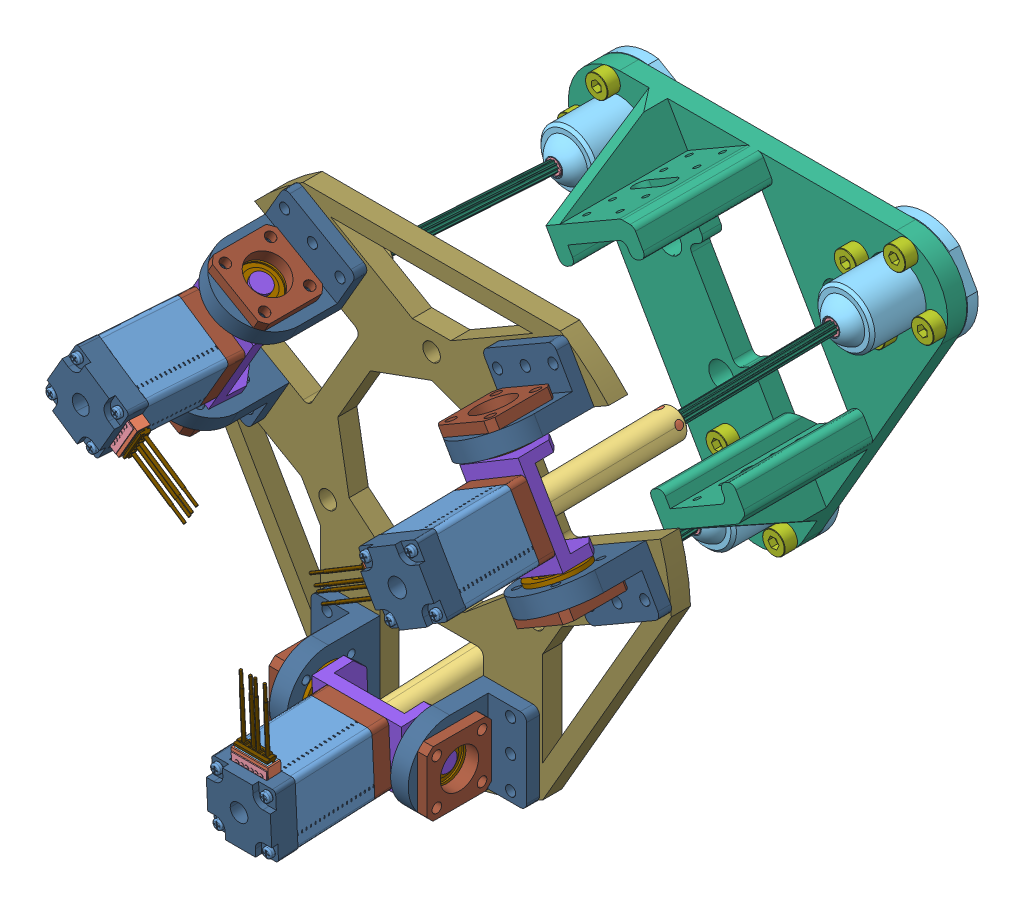
SolidWorks assembly 人形机器人脖子, configuration 默认. Lengths in mm.
Overall size (162.55 157.59 172.71).
143 component instances, 31 part files, 94 mates.
Components (placement in the parent):
- 20K-2M..50-1: 20K-2M..50 [默认] at (-49.4711 28.5622 60.199) x (0.041576 -0.024004 -0.998847) z (-0.865027 0.499423 -0.048008) size (146.95 25.88 47.14)
  - 20K-2M..50.STEP-1: 20K-2M..50.STEP [默认] at origin size (146.95 25.88 47.14)
    - 02-20-42.STEP-1: 02-20-42.STEP [默认] at (19.975 0 0) x (0 -1 0) z (-1 0 0) size (25.88 26.04 31.85)
      - 02-20-24.15_10-20-001-2.STEP-1: 02-20-24.15_10-20-001-2.STEP [默认] at origin size (20 20 24.15)
      - 13-20-12.5____.STEP-1: 13-20-12.5____.STEP [默认] at (0 0 16.075) x (-1 0 0) z (0 0 -1) size (18.2 22.2 16.51)
      - 13-20-12.5______.STEP-1: 13-20-12.5______.STEP [默认] at (0 0 -14.575) x (0.707107 0.707107 0) z (0 0 1) size (18.3 18.3 15.8)
      - 20-20__________.STEP-1: 20-20__________.STEP [默认] at (0 0 15.675) size (17.8 21 0.9)
      - 13-20-001________.STEP-1: 13-20-001________.STEP [默认] at (0 -8.6 12.175) x (1 0 0) z (0 0 -1) size (10.5 7.2 3.5)
    - 03-20-006____42_____default.STEP-1: 03-20-006____42_____default.STEP [默认] at (5.7 0 0) x (1 0 0) z (0 0.381126 -0.924523) size (29.65 16.26 16.27)
      - 06-20-006____42______YK_01-20-007-1.STEP-1: 06-20-006____42______YK_01-20-007-1.STEP [默认] at origin size (29.65 7 7)
      - 03-20-4.2-6YK_10-20-006-2.STEP-1: 03-20-4.2-6YK_10-20-006-2.STEP [默认] at (22.53 0 0) x (0 0.91534 0.402682) z (-1 0 0) size (12.06 12.08 4.24)
      - 10-20-001__________.STEP-1: 10-20-001__________.STEP [默认] at (14.67 0 0) x (0 0 1) z (-1 0 0) size (11 11 1)
      - 08-20-001_____07-20-001-1.STEP-1: 08-20-001_____07-20-001-1.STEP [默认] at (20.41 0 0) x (0 0 1) z (-1 0 0) size (11 11 1.5)
      - 08-20-001_____07-20-001-1.STEP-2: 08-20-001_____07-20-001-1.STEP [默认] at (9.43 0 0) x (0 0 1) z (-1 0 0) size (11 11 1.5)
      - 03-20-4.2-6YK_10-20-006-2.STEP-2: 03-20-4.2-6YK_10-20-006-2.STEP [默认] at (16.79 0 0) x (0 0.888249 0.459362) z (-1 0 0) size (12.06 12.08 4.24)
      - 03-20-4.2-6YK_10-20-006-2.STEP-3: 03-20-4.2-6YK_10-20-006-2.STEP [默认] at (11.55 0 0) x (0 0.91534 0.402682) z (-1 0 0) size (12.06 12.08 4.24)
      - 03-20-4.2-6YK_10-20-006-2.STEP-4: 03-20-4.2-6YK_10-20-006-2.STEP [默认] at (5.81 0 0) x (0 0.888249 0.459362) z (-1 0 0) size (12.06 12.08 4.24)
    - 01-20-006__20__________YK__.STEP-1: 01-20-006__20__________YK__.STEP [默认] at origin size (8.8 20 20)
    - 01-20-005(20____________YK__.STEP-1: 01-20-005(20____________YK__.STEP [默认] at (31.25 0 0) x (0 0 -1) z (1 0 0) size (20 20 7.5)
    - 09-20-001____9X__5X4)_09-20-001.STEP-1: 09-20-001____9X__5X4)_09-20-001.STEP [默认] at (5.7 0 0) x (1 0 0) z (0 0.998527 -0.054257) size (3 9 9)
    - 09-20-001____9X__5X4)_09-20-001.STEP-2: 09-20-001____9X__5X4)_09-20-001.STEP [默认] at (32.35 0 0) x (1 0 0) z (0 0.945037 0.326964) size (3 9 9)
    - 06-20-017__20________YK___20____________YK.STEP-1: 06-20-017__20________YK___20____________YK.STEP [默认] at (30.35 0 0) x (0 0.924523 0.381126) z (-1 0 0) size (6.01 6.01 10)
    - 07-20-007__________________.STEP-1: 07-20-007__________________.STEP [默认] at (38.75 0 0) x (-1 0 0) z (0 -0.999857 -0.016895) size (6 12.92 13)
    - 07-20-015-1______________.STEP-1: 07-20-015-1______________.STEP [默认] at (82.15 0 0) x (0 -0.714016 0.700129) z (1 0 0) size (3.42 3.5 64.8)
    - 07-20-015-2______________.STEP-1: 07-20-015-2______________.STEP [默认] at (20.35 0 0) x (0 0.924225 0.381849) z (1 0 0) size (3.5 3.9 64.81)
    - 07-20-006__20______.STEP-1: 07-20-006__20______.STEP [默认] at (86.15 0 0) x (0 0.924225 0.381849) z (1 0 0) size (3.9 4.45 0.4)
    - 14-20-001__20-28____________________.STEP-1: 14-20-001__20-28____________________.STEP [默认] at (6.48 -0.2 -10) x (0 -1 0) z (0 0 1) size (10.5 3.4 24.5)
    - 11-20-001__M2-24.5__20-30__.STEP-1: 11-20-001__M2-24.5__20-30__.STEP [默认] at (0.39 7.7 -7.7) x (0 -0.010787 -0.999942) z (1 0 0) size (3 3 26)
    - 11-20-001__M2-24.5__20-30__.STEP-2: 11-20-001__M2-24.5__20-30__.STEP [默认] at (0.39 7.7 7.7) x (0 0.999942 -0.010787) z (1 0 0) size (3 3 26)
    - 11-20-001__M2-24.5__20-30__.STEP-3: 11-20-001__M2-24.5__20-30__.STEP [默认] at (0.39 -7.7 7.7) x (0 0.010787 0.999942) z (1 0 0) size (3 3 26)
    - 11-20-001__M2-24.5__20-30__.STEP-4: 11-20-001__M2-24.5__20-30__.STEP [默认] at (0.39 -7.7 -7.7) x (0 -0.999942 0.010787) z (1 0 0) size (3 3 26)
    - 07-20-002__20________________.STEP-1: 07-20-002__20________________.STEP [默认] at (87.8 0 0) x (0 0 -1) z (1 0 0) size (9.01 9.01 3.1)
    - 07-20-015-3__20_____________08-20-002-1.STEP-1: 07-20-015-3__20_____________08-20-002-1.STEP [默认] at (35.35 0 0) x (0 0 -1) z (1 0 0) size (9.01 9.01 54.8)
- 螺纹转换套-1: 螺纹转换套 [默认] at (-43.3616 25.0348 -86.5816) x (-0.216556 -0.976163 0.014445) z (-0.041576 0.024004 0.998847) size (5 5 5)
- 球铰-1: 球铰 [默认] at (-43.3013 25 -111.5299) x (-0.5 -0.866025 0) z (-0.866025 0.5 0) size (30 29.95 32)
- 球-1: 球 [默认] at (-43.3013 25 -88.0299) x (-0.689413 -0.72428 -0.01129) z (0.723174 -0.689088 0.046661) size (14 13.45 14) (hidden)
- 20K-2M..50-2: 20K-2M..50 [默认] at (49.4711 28.5622 60.199) x (-0.041576 -0.024004 -0.998847) z (0.865027 0.499423 -0.048008) size (146.95 25.88 47.14)
  - 20K-2M..50.STEP-1: 20K-2M..50.STEP [默认] at origin size (146.95 25.88 47.14)
    - 02-20-42.STEP-1: 02-20-42.STEP [默认] at (19.975 0 0) x (0 -1 0) z (-1 0 0) size (25.88 26.04 31.85)
      - 02-20-24.15_10-20-001-2.STEP-1: 02-20-24.15_10-20-001-2.STEP [默认] at origin size (20 20 24.15)
      - 13-20-12.5____.STEP-1: 13-20-12.5____.STEP [默认] at (0 0 16.075) x (-1 0 0) z (0 0 -1) size (18.2 22.2 16.51)
      - 13-20-12.5______.STEP-1: 13-20-12.5______.STEP [默认] at (0 0 -14.575) x (0.707107 0.707107 0) z (0 0 1) size (18.3 18.3 15.8)
      - 20-20__________.STEP-1: 20-20__________.STEP [默认] at (0 0 15.675) size (17.8 21 0.9)
      - 13-20-001________.STEP-1: 13-20-001________.STEP [默认] at (0 -8.6 12.175) x (1 0 0) z (0 0 -1) size (10.5 7.2 3.5)
    - 03-20-006____42_____default.STEP-1: 03-20-006____42_____default.STEP [默认] at (5.7 0 0) x (1 0 0) z (0 0.381126 -0.924523) size (29.65 16.26 16.27)
      - 06-20-006____42______YK_01-20-007-1.STEP-1: 06-20-006____42______YK_01-20-007-1.STEP [默认] at origin size (29.65 7 7)
      - 03-20-4.2-6YK_10-20-006-2.STEP-1: 03-20-4.2-6YK_10-20-006-2.STEP [默认] at (22.53 0 0) x (0 0.91534 0.402682) z (-1 0 0) size (12.06 12.08 4.24)
      - 10-20-001__________.STEP-1: 10-20-001__________.STEP [默认] at (14.67 0 0) x (0 0 1) z (-1 0 0) size (11 11 1)
      - 08-20-001_____07-20-001-1.STEP-1: 08-20-001_____07-20-001-1.STEP [默认] at (20.41 0 0) x (0 0 1) z (-1 0 0) size (11 11 1.5)
      - 08-20-001_____07-20-001-1.STEP-2: 08-20-001_____07-20-001-1.STEP [默认] at (9.43 0 0) x (0 0 1) z (-1 0 0) size (11 11 1.5)
      - 03-20-4.2-6YK_10-20-006-2.STEP-2: 03-20-4.2-6YK_10-20-006-2.STEP [默认] at (16.79 0 0) x (0 0.888249 0.459362) z (-1 0 0) size (12.06 12.08 4.24)
      - 03-20-4.2-6YK_10-20-006-2.STEP-3: 03-20-4.2-6YK_10-20-006-2.STEP [默认] at (11.55 0 0) x (0 0.91534 0.402682) z (-1 0 0) size (12.06 12.08 4.24)
      - 03-20-4.2-6YK_10-20-006-2.STEP-4: 03-20-4.2-6YK_10-20-006-2.STEP [默认] at (5.81 0 0) x (0 0.888249 0.459362) z (-1 0 0) size (12.06 12.08 4.24)
    - 01-20-006__20__________YK__.STEP-1: 01-20-006__20__________YK__.STEP [默认] at origin size (8.8 20 20)
    - 01-20-005(20____________YK__.STEP-1: 01-20-005(20____________YK__.STEP [默认] at (31.25 0 0) x (0 0 -1) z (1 0 0) size (20 20 7.5)
    - 09-20-001____9X__5X4)_09-20-001.STEP-1: 09-20-001____9X__5X4)_09-20-001.STEP [默认] at (5.7 0 0) x (1 0 0) z (0 0.998527 -0.054257) size (3 9 9)
    - 09-20-001____9X__5X4)_09-20-001.STEP-2: 09-20-001____9X__5X4)_09-20-001.STEP [默认] at (32.35 0 0) x (1 0 0) z (0 0.945037 0.326964) size (3 9 9)
    - 06-20-017__20________YK___20____________YK.STEP-1: 06-20-017__20________YK___20____________YK.STEP [默认] at (30.35 0 0) x (0 0.924523 0.381126) z (-1 0 0) size (6.01 6.01 10)
    - 07-20-007__________________.STEP-1: 07-20-007__________________.STEP [默认] at (38.75 0 0) x (-1 0 0) z (0 -0.999857 -0.016895) size (6 12.92 13)
    - 07-20-015-1______________.STEP-1: 07-20-015-1______________.STEP [默认] at (82.15 0 0) x (0 -0.714016 0.700129) z (1 0 0) size (3.42 3.5 64.8)
    - 07-20-015-2______________.STEP-1: 07-20-015-2______________.STEP [默认] at (20.35 0 0) x (0 0.924225 0.381849) z (1 0 0) size (3.5 3.9 64.81)
    - 07-20-006__20______.STEP-1: 07-20-006__20______.STEP [默认] at (86.15 0 0) x (0 0.924225 0.381849) z (1 0 0) size (3.9 4.45 0.4)
    - 14-20-001__20-28____________________.STEP-1: 14-20-001__20-28____________________.STEP [默认] at (6.48 -0.2 -10) x (0 -1 0) z (0 0 1) size (10.5 3.4 24.5)
    - 11-20-001__M2-24.5__20-30__.STEP-1: 11-20-001__M2-24.5__20-30__.STEP [默认] at (0.39 7.7 -7.7) x (0 -0.010787 -0.999942) z (1 0 0) size (3 3 26)
    - 11-20-001__M2-24.5__20-30__.STEP-2: 11-20-001__M2-24.5__20-30__.STEP [默认] at (0.39 7.7 7.7) x (0 0.999942 -0.010787) z (1 0 0) size (3 3 26)
    - 11-20-001__M2-24.5__20-30__.STEP-3: 11-20-001__M2-24.5__20-30__.STEP [默认] at (0.39 -7.7 7.7) x (0 0.010787 0.999942) z (1 0 0) size (3 3 26)
    - 11-20-001__M2-24.5__20-30__.STEP-4: 11-20-001__M2-24.5__20-30__.STEP [默认] at (0.39 -7.7 -7.7) x (0 -0.999942 0.010787) z (1 0 0) size (3 3 26)
    - 07-20-002__20________________.STEP-1: 07-20-002__20________________.STEP [默认] at (87.8 0 0) x (0 0 -1) z (1 0 0) size (9.01 9.01 3.1)
    - 07-20-015-3__20_____________08-20-002-1.STEP-1: 07-20-015-3__20_____________08-20-002-1.STEP [默认] at (35.35 0 0) x (0 0 -1) z (1 0 0) size (9.01 9.01 54.8)
- 20K-2M..50-3: 20K-2M..50 [默认] at (0 -57.1243 60.199) x (0 0.048008 -0.998847) z (0 -0.998847 -0.048008) size (146.95 25.88 47.14)
  - 20K-2M..50.STEP-1: 20K-2M..50.STEP [默认] at origin size (146.95 25.88 47.14)
    - 02-20-42.STEP-1: 02-20-42.STEP [默认] at (19.975 0 0) x (0 -1 0) z (-1 0 0) size (25.88 26.04 31.85)
      - 02-20-24.15_10-20-001-2.STEP-1: 02-20-24.15_10-20-001-2.STEP [默认] at origin size (20 20 24.15)
      - 13-20-12.5____.STEP-1: 13-20-12.5____.STEP [默认] at (0 0 16.075) x (-1 0 0) z (0 0 -1) size (18.2 22.2 16.51)
      - 13-20-12.5______.STEP-1: 13-20-12.5______.STEP [默认] at (0 0 -14.575) x (0.707107 0.707107 0) z (0 0 1) size (18.3 18.3 15.8)
      - 20-20__________.STEP-1: 20-20__________.STEP [默认] at (0 0 15.675) size (17.8 21 0.9)
      - 13-20-001________.STEP-1: 13-20-001________.STEP [默认] at (0 -8.6 12.175) x (1 0 0) z (0 0 -1) size (10.5 7.2 3.5)
    - 03-20-006____42_____default.STEP-1: 03-20-006____42_____default.STEP [默认] at (5.7 0 0) x (1 0 0) z (0 0.381126 -0.924523) size (29.65 16.26 16.27)
      - 06-20-006____42______YK_01-20-007-1.STEP-1: 06-20-006____42______YK_01-20-007-1.STEP [默认] at origin size (29.65 7 7)
      - 03-20-4.2-6YK_10-20-006-2.STEP-1: 03-20-4.2-6YK_10-20-006-2.STEP [默认] at (22.53 0 0) x (0 0.91534 0.402682) z (-1 0 0) size (12.06 12.08 4.24)
      - 10-20-001__________.STEP-1: 10-20-001__________.STEP [默认] at (14.67 0 0) x (0 0 1) z (-1 0 0) size (11 11 1)
      - 08-20-001_____07-20-001-1.STEP-1: 08-20-001_____07-20-001-1.STEP [默认] at (20.41 0 0) x (0 0 1) z (-1 0 0) size (11 11 1.5)
      - 08-20-001_____07-20-001-1.STEP-2: 08-20-001_____07-20-001-1.STEP [默认] at (9.43 0 0) x (0 0 1) z (-1 0 0) size (11 11 1.5)
      - 03-20-4.2-6YK_10-20-006-2.STEP-2: 03-20-4.2-6YK_10-20-006-2.STEP [默认] at (16.79 0 0) x (0 0.888249 0.459362) z (-1 0 0) size (12.06 12.08 4.24)
      - 03-20-4.2-6YK_10-20-006-2.STEP-3: 03-20-4.2-6YK_10-20-006-2.STEP [默认] at (11.55 0 0) x (0 0.91534 0.402682) z (-1 0 0) size (12.06 12.08 4.24)
      - 03-20-4.2-6YK_10-20-006-2.STEP-4: 03-20-4.2-6YK_10-20-006-2.STEP [默认] at (5.81 0 0) x (0 0.888249 0.459362) z (-1 0 0) size (12.06 12.08 4.24)
    - 01-20-006__20__________YK__.STEP-1: 01-20-006__20__________YK__.STEP [默认] at origin size (8.8 20 20)
    - 01-20-005(20____________YK__.STEP-1: 01-20-005(20____________YK__.STEP [默认] at (31.25 0 0) x (0 0 -1) z (1 0 0) size (20 20 7.5)
    - 09-20-001____9X__5X4)_09-20-001.STEP-1: 09-20-001____9X__5X4)_09-20-001.STEP [默认] at (5.7 0 0) x (1 0 0) z (0 0.998527 -0.054257) size (3 9 9)
    - 09-20-001____9X__5X4)_09-20-001.STEP-2: 09-20-001____9X__5X4)_09-20-001.STEP [默认] at (32.35 0 0) x (1 0 0) z (0 0.945037 0.326964) size (3 9 9)
    - 06-20-017__20________YK___20____________YK.STEP-1: 06-20-017__20________YK___20____________YK.STEP [默认] at (30.35 0 0) x (0 0.924523 0.381126) z (-1 0 0) size (6.01 6.01 10)
    - 07-20-007__________________.STEP-1: 07-20-007__________________.STEP [默认] at (38.75 0 0) x (-1 0 0) z (0 -0.999857 -0.016895) size (6 12.92 13)
    - 07-20-015-1______________.STEP-1: 07-20-015-1______________.STEP [默认] at (82.15 0 0) x (0 -0.714016 0.700129) z (1 0 0) size (3.42 3.5 64.8)
    - 07-20-015-2______________.STEP-1: 07-20-015-2______________.STEP [默认] at (20.35 0 0) x (0 0.924225 0.381849) z (1 0 0) size (3.5 3.9 64.81)
    - 07-20-006__20______.STEP-1: 07-20-006__20______.STEP [默认] at (86.15 0 0) x (0 0.924225 0.381849) z (1 0 0) size (3.9 4.45 0.4)
    - 14-20-001__20-28____________________.STEP-1: 14-20-001__20-28____________________.STEP [默认] at (6.48 -0.2 -10) x (0 -1 0) z (0 0 1) size (10.5 3.4 24.5)
    - 11-20-001__M2-24.5__20-30__.STEP-1: 11-20-001__M2-24.5__20-30__.STEP [默认] at (0.39 7.7 -7.7) x (0 -0.010787 -0.999942) z (1 0 0) size (3 3 26)
    - 11-20-001__M2-24.5__20-30__.STEP-2: 11-20-001__M2-24.5__20-30__.STEP [默认] at (0.39 7.7 7.7) x (0 0.999942 -0.010787) z (1 0 0) size (3 3 26)
    - 11-20-001__M2-24.5__20-30__.STEP-3: 11-20-001__M2-24.5__20-30__.STEP [默认] at (0.39 -7.7 7.7) x (0 0.010787 0.999942) z (1 0 0) size (3 3 26)
    - 11-20-001__M2-24.5__20-30__.STEP-4: 11-20-001__M2-24.5__20-30__.STEP [默认] at (0.39 -7.7 -7.7) x (0 -0.999942 0.010787) z (1 0 0) size (3 3 26)
    - 07-20-002__20________________.STEP-1: 07-20-002__20________________.STEP [默认] at (87.8 0 0) x (0 0 -1) z (1 0 0) size (9.01 9.01 3.1)
    - 07-20-015-3__20_____________08-20-002-1.STEP-1: 07-20-015-3__20_____________08-20-002-1.STEP [默认] at (35.35 0 0) x (0 0 -1) z (1 0 0) size (9.01 9.01 54.8)
- 螺纹转换套-2: 螺纹转换套 [默认] at (43.5694 25.1548 -81.5873) x (0.764019 -0.644988 -0.016301) z (-0.041576 -0.024004 -0.998847) size (5 5 5)
- 螺纹转换套-3: 螺纹转换套 [默认] at (0 -50.3096 -81.5873) x (0.533096 0.845079 0.040617) z (0 0.048008 -0.998847) size (5 5 5)
- 球铰-2: 球铰 [默认] at (0 -50 -111.5299) x (0 -1 0) z (-1 0 0) size (30 29.95 32)
- 球铰-3: 球铰 [默认] at (43.3013 25 -111.5299) x (-0.866025 -0.5 0) z (-0.5 0.866025 0) size (30 29.95 32)
- 球-2: 球 [默认] at (0 -50 -88.0299) x (-0.99893 -0.046188 -0.00222) z (0.046242 -0.997778 -0.047956) size (14 13.45 14) (hidden)
- 球-3: 球 [默认] at (43.3013 25 -88.0299) x (0.893401 -0.448483 -0.026409) z (0.447332 0.893469 -0.040091) size (14 13.45 14) (hidden)
- 云台-1: 云台 [默认] at (0 0 -102.0299) x (-0.5 0.866025 0) z (0 0 -1) size (118.6 107 46)
- TCBAS通孔型内六角螺栓[TCBAS4-10]-1: TCBAS通孔型内六角螺栓[TCBAS4-10] [TCBAS4-10] at (-55.3753 21.7648 -98.0299) x (-0.412704 -0.910865 0) z (-0.910865 0.412704 0) size (7 14 7)
- TCBAS通孔型内六角螺栓[TCBAS4-10]-2: TCBAS通孔型内六角螺栓[TCBAS4-10] [TCBAS4-10] at (-40.066 12.9259 -98.0299) x (0.910865 -0.412704 0) z (-0.412704 -0.910865 0) size (7 14 7)
- TCBAS通孔型内六角螺栓[TCBAS4-10]-3: TCBAS通孔型内六角螺栓[TCBAS4-10] [TCBAS4-10] at (-31.2272 28.2352 -98.0299) x (0.412704 0.910865 0) z (0.910865 -0.412704 0) size (7 14 7)
- TCBAS通孔型内六角螺栓[TCBAS4-10]-4: TCBAS通孔型内六角螺栓[TCBAS4-10] [TCBAS4-10] at (-46.5365 37.0741 -98.0299) x (-0.910865 0.412704 0) z (0.412704 0.910865 0) size (7 14 7)
- TCBAS通孔型内六角螺栓[TCBAS4-10]-5: TCBAS通孔型内六角螺栓[TCBAS4-10] [TCBAS4-10] at (8.8388 -58.8388 -98.0299) x (0.995184 0.098021 0) z (0.098021 -0.995184 0) size (7 14 7)
- TCBAS通孔型内六角螺栓[TCBAS4-10]-6: TCBAS通孔型内六角螺栓[TCBAS4-10] [TCBAS4-10] at (46.5365 37.0741 -98.0299) x (-0.582481 0.812845 0) z (0.812845 0.582481 0) size (7 14 7)
- TCBAS通孔型内六角螺栓[TCBAS4-10]-7: TCBAS通孔型内六角螺栓[TCBAS4-10] [TCBAS4-10] at (8.8388 -41.1612 -98.0299) x (-0.098021 0.995184 0) z (0.995184 0.098021 0) size (7 14 7)
- TCBAS通孔型内六角螺栓[TCBAS4-10]-8: TCBAS通孔型内六角螺栓[TCBAS4-10] [TCBAS4-10] at (31.2272 28.2352 -98.0299) x (-0.812845 -0.582481 0) z (-0.582481 0.812845 0) size (7 14 7)
- TCBAS通孔型内六角螺栓[TCBAS4-10]-9: TCBAS通孔型内六角螺栓[TCBAS4-10] [TCBAS4-10] at (-8.8388 -41.1612 -98.0299) x (-0.995184 -0.098021 0) z (-0.098021 0.995184 0) size (7 14 7)
- TCBAS通孔型内六角螺栓[TCBAS4-10]-10: TCBAS通孔型内六角螺栓[TCBAS4-10] [TCBAS4-10] at (40.066 12.9259 -98.0299) x (0.582481 -0.812845 0) z (-0.812845 -0.582481 0) size (7 14 7)
- TCBAS通孔型内六角螺栓[TCBAS4-10]-11: TCBAS通孔型内六角螺栓[TCBAS4-10] [TCBAS4-10] at (-8.8388 -58.8388 -98.0299) x (0.098021 -0.995184 0) z (-0.995184 -0.098021 0) size (7 14 7)
- TCBAS通孔型内六角螺栓[TCBAS4-10]-12: TCBAS通孔型内六角螺栓[TCBAS4-10] [TCBAS4-10] at (55.3753 21.7648 -98.0299) x (0.812845 0.582481 0) z (0.582481 -0.812845 0) size (7 14 7)
- 电缸座-1: 电缸座 [默认] at (47.9224 27.668 22.9919) x (-0.5 0.866025 0) z (-0.041576 -0.024004 -0.998847) size (42 20 14)
- F696.ZZ-1: F696.ZZ [默认] at (55.1314 14.5096 16) x (-0.801441 -0.462712 -0.378931) z (-0.328164 -0.189466 0.925425) size (17 5 17)
- F696.ZZ-2: F696.ZZ [默认] at (40.1314 40.4904 16) x (0.852847 0.492391 -0.17379) z (0.150506 0.086895 0.984783) size (17 5 17)
- 回转座-1: 回转座 [默认] at (55.7314 13.4704 16) x (0.866025 0.5 0) z (0.5 -0.866025 0) size (26 29 17.5)
- 回转座-2: 回转座 [默认] at (39.5314 41.5296 16) x (-0.866025 -0.5 0) z (-0.5 0.866025 0) size (26 29 17.5)
- 轴承端盖-1: 轴承端盖 [默认] at (59.9814 6.1092 16) x (0 0 1) z (-0.5 0.866025 0) size (20.14 20.14 4)
- 轴承端盖-2: 轴承端盖 [默认] at (35.2814 48.8908 16) x (0 0 1) z (0.5 -0.866025 0) size (20.14 20.14 4)
- 打磨系统法兰改-1: 打磨系统法兰改 [默认] x (-1 0 0) z (0 0 -1) size (149.86 136.53 6)
- 电缸座-4: 电缸座 [默认] at (0 -55.3361 22.9919) x (-1 0 0) z (0 0.048008 -0.998847) size (42 20 14)
- 电缸座-5: 电缸座 [默认] at (-47.9224 27.668 22.9919) x (0.5 0.866025 0) z (0.041576 -0.024004 -0.998847) size (42 20 14)
- 回转座-7: 回转座 [默认] at (-39.5314 41.5296 16) x (-0.866025 0.5 0) z (0.5 0.866025 0) size (26 29 17.5)
- 回转座-8: 回转座 [默认] at (-55.7314 13.4704 16) x (0.866025 -0.5 0) z (-0.5 -0.866025 0) size (26 29 17.5)
- 回转座-9: 回转座 [默认] at (-16.2 -55 16) x (0 -1 0) z (-1 0 0) size (26 29 17.5)
- 回转座-10: 回转座 [默认] at (16.2 -55 16) x (0 1 0) z (1 0 0) size (26 29 17.5)
- F696.ZZ-7: F696.ZZ [默认] at (-40.1314 40.4904 16) x (0.814397 -0.470192 0.340113) z (-0.294546 0.170056 0.940385) size (17 5 17)
- F696.ZZ-8: F696.ZZ [默认] at (-55.1314 14.5096 16) x (-0.801441 0.462712 -0.378931) z (-0.328164 0.189466 0.925425) size (17 5 17)
- F696.ZZ-9: F696.ZZ [默认] at (-15 -55 16) x (0 -0.003155 0.999995) z (0 -0.999995 -0.003155) size (17 5 17)
- F696.ZZ-10: F696.ZZ [默认] at (15 -55 16) x (0 -0.925425 -0.378931) z (0 -0.378931 0.925425) size (17 5 17)
- 轴承端盖-7: 轴承端盖 [默认] at (24.7 -55 16) x (0 0 1) z (-1 0 0) size (20.14 20.14 4)
- 轴承端盖-8: 轴承端盖 [默认] at (-24.7 -55 16) x (0 -1 0) z (1 0 0) size (20.14 20.14 4)
- 轴承端盖-9: 轴承端盖 [默认] at (-59.9814 6.1092 16) x (0 0 1) z (0.5 0.866025 0) size (20.14 20.14 4)
- 轴承端盖-10: 轴承端盖 [默认] at (-35.2814 48.8908 16) x (0 0 1) z (-0.5 -0.866025 0) size (20.14 20.14 4)
Mates (geometry in assembly coordinates):
- 距离3: distance = 0 mm anti-aligned: plane of 20K-2M..50-1/20K-2M..50.STEP-1/07-20-015-1______________.STEP-1 through (-43.5694 25.1548 -81.5873) normal (0.041576 -0.024004 -0.998847); plane of 螺纹转换套-1 through (-43.5694 25.1548 -81.5873) normal (-0.041576 0.024004 0.998847)
- 同心1: concentric aligned: cylinder of 20K-2M..50-1/20K-2M..50.STEP-1/07-20-015-1______________.STEP-1 through (-43.5694 25.1548 -81.5873) axis (0.041576 -0.024004 -0.998847) radius 1.25; cylinder of 螺纹转换套-1 through (-43.5694 25.1548 -81.5873) axis (0.041576 -0.024004 -0.998847) radius 1.25
- 同心4: concentric anti-aligned: cylinder of 螺纹转换套-1 through (-43.5694 25.1548 -81.5873) axis (0.041576 -0.024004 -0.998847) radius 2.5; cylinder of 球-1 through (-43.3616 25.0348 -86.5816) axis (-0.041576 0.024004 0.998847) radius 2.5
- 同心6: concentric anti-aligned: cylinder of 20K-2M..50-2/20K-2M..50.STEP-1/07-20-015-1______________.STEP-1 through (43.5694 25.1548 -81.5873) axis (-0.041576 -0.024004 -0.998847) radius 1.25; circle of 球-3
- 同心7: concentric aligned: cylinder of 螺纹转换套-2 through (43.3616 25.0348 -86.5816) axis (0.041576 0.024004 0.998847) radius 2.5; cylinder of 球-3 through (43.3616 25.0348 -86.5816) axis (0.041576 0.024004 0.998847) radius 2.5
- 重合5: coincident anti-aligned: plane of 螺纹转换套-2 through (43.3616 25.0348 -86.5816) normal (-0.041576 -0.024004 -0.998847); plane of 球-3 through (43.3616 25.0348 -86.5816) normal (0.041576 0.024004 0.998847)
- 重合6: coincident anti-aligned: plane of 螺纹转换套-3 through (0 -50.0696 -86.5816) normal (0 0.048008 -0.998847); plane of 球-2 through (0 -50.0696 -86.5816) normal (0 -0.048008 0.998847)
- 同心8: concentric aligned: cylinder of 螺纹转换套-3 through (0 -50.0696 -86.5816) axis (0 -0.048008 0.998847) radius 2.5; cylinder of 球-2 through (0 -50.0696 -86.5816) axis (0 -0.048008 0.998847) radius 2.5
- 距离4: distance = 0 mm anti-aligned: plane of 20K-2M..50-3/20K-2M..50.STEP-1/07-20-015-1______________.STEP-1 through (0 -50.3096 -81.5873) normal (0 0.048008 -0.998847); plane of 螺纹转换套-3 through (0 -50.3096 -81.5873) normal (0 -0.048008 0.998847)
- 同心9: concentric anti-aligned: cylinder of 20K-2M..50-3/20K-2M..50.STEP-1/07-20-015-1______________.STEP-1 through (0 -50.3096 -81.5873) axis (0 0.048008 -0.998847) radius 1.25; cylinder of 螺纹转换套-3 through (0 -50.0696 -86.5816) axis (0 -0.048008 0.998847) radius 1.25
- 同心11: concentric: sphere of 球铰-3; sphere of 球-3
- 重合19: coincident anti-aligned: plane of 球铰-1 through (-51.3013 11.1436 -108.0299) normal (0 0 1); plane of 云台-1 through (0 0 -108.0299) normal (0 0 -1)
- 重合20: coincident anti-aligned: plane of 球铰-3 through (29.4449 17 -108.0299) normal (0 0 1); plane of 云台-1 through (0 0 -108.0299) normal (0 0 -1)
- 重合21: coincident anti-aligned: plane of 球铰-2 through (0 -66 -108.0299) normal (0 0 1); plane of 云台-1 through (0 0 -108.0299) normal (0 0 -1)
- 同心23: concentric anti-aligned: cylinder of 球铰-2 through (-8.8388 -58.8388 -113.0299) axis (0 0 1) radius 2; cylinder of 云台-1 through (-8.8388 -58.8388 -102.0299) axis (0 0 -1) radius 2
- 同心24: concentric anti-aligned: cylinder of 球铰-2 through (-8.8388 -41.1612 -113.0299) axis (0 0 1) radius 2; cylinder of 云台-1 through (-8.8388 -41.1612 -102.0299) axis (0 0 -1) radius 2
- 重合22: coincident anti-aligned: cylinder of 球铰-1 through (-46.5365 37.0741 -113.0299) axis (0 0 1) radius 2; circle of 云台-1
- 同心25: concentric anti-aligned: cylinder of 球铰-1 through (-31.2272 28.2352 -113.0299) axis (0 0 1) radius 2; cylinder of 云台-1 through (-31.2272 28.2352 -102.0299) axis (0 0 -1) radius 2
- 同心26: concentric anti-aligned: cylinder of 球铰-3 through (55.3753 21.7648 -113.0299) axis (0 0 1) radius 2; cylinder of 云台-1 through (55.3753 21.7648 -102.0299) axis (0 0 -1) radius 2
- 同心27: concentric anti-aligned: cylinder of 球铰-3 through (46.5365 37.0741 -113.0299) axis (0 0 1) radius 2; cylinder of 云台-1 through (46.5365 37.0741 -102.0299) axis (0 0 -1) radius 2
- 同心28: concentric anti-aligned: cylinder of 云台-1 through (-55.3753 21.7648 -102.0299) axis (0 0 -1) radius 2; cylinder of TCBAS通孔型内六角螺栓[TCBAS4-10]-1 through (-55.3753 21.7648 -100.8959) axis (0 0 1) radius 2
- 重合25: coincident anti-aligned: plane of 云台-1 through (0 0 -102.0299) normal (0 0 1); plane of TCBAS通孔型内六角螺栓[TCBAS4-10]-1 through (-56.2008 19.943 -102.0299) normal (0 0 -1)
- 同心45: concentric anti-aligned: cylinder of 20K-2M..50-2/20K-2M..50.STEP-1/01-20-005(20____________YK__.STEP-1 through (47.9224 27.668 22.9919) axis (-0.041576 -0.024004 -0.998847) radius 8; cylinder of 电缸座-1 through (47.7561 27.572 18.9965) axis (0.041576 0.024004 0.998847) radius 8
- 重合39: coincident anti-aligned: plane of 20K-2M..50-2/20K-2M..50.STEP-1/01-20-005(20____________YK__.STEP-1 through (36.3197 30.7841 23.4) normal (-0.041576 -0.024004 -0.998847); plane of 电缸座-1 through (47.9224 27.668 22.9919) normal (0.041576 0.024004 0.998847)
- 同心47: concentric aligned: cylinder of 20K-2M..50-2/20K-2M..50.STEP-1/01-20-005(20____________YK__.STEP-1 through (45.0494 17.1181 21.8633) axis (0.041576 0.024004 0.998847) radius 0.75; cylinder of 电缸座-1 through (44.9454 17.0581 19.3662) axis (0.041576 0.024004 0.998847) radius 1
- 同心48: concentric anti-aligned: cylinder of 电缸座-1 through (58.1314 9.3135 16) axis (-0.5 0.866025 0) radius 3; cylinder of F696.ZZ-1 through (58.7361 8.2661 16) axis (0.5 -0.866025 0) radius 7.5
- 重合40: coincident anti-aligned: plane of 电缸座-1 through (55.4224 14.6776 22.9919) normal (0.5 -0.866025 0); plane of F696.ZZ-1 through (51.5249 12.4274 14.2948) normal (-0.5 0.866025 0)
- 重合41: coincident anti-aligned: plane of 电缸座-1 through (40.4224 40.6584 22.9919) normal (-0.5 0.866025 0); plane of F696.ZZ-2 through (43.9692 42.7061 15.2179) normal (0.5 -0.866025 0)
- 同心49: concentric anti-aligned: cylinder of 电缸座-1 through (37.1314 45.6865 16) axis (0.5 -0.866025 0) radius 3; cylinder of F696.ZZ-2 through (36.5267 46.7339 16) axis (-0.5 0.866025 0) radius 3
- 同心50: concentric anti-aligned: cylinder of F696.ZZ-1 through (58.7361 8.2661 16) axis (0.5 -0.866025 0) radius 7.5; cylinder of 回转座-1 through (58.4814 8.7072 16) axis (-0.5 0.866025 0) radius 7.5
- 同心51: concentric anti-aligned: cylinder of F696.ZZ-2 through (36.5267 46.7339 16) axis (-0.5 0.866025 0) radius 7.5; cylinder of 回转座-2 through (36.7814 46.2928 16) axis (0.5 -0.866025 0) radius 7.5
- 重合42: coincident anti-aligned: plane of F696.ZZ-2 through (45.9277 45.2225 14.6966) normal (-0.5 0.866025 0); plane of 回转座-2 through (39.5314 41.5296 16) normal (0.5 -0.866025 0)
- 重合43: coincident anti-aligned: plane of F696.ZZ-1 through (49.7206 10 13.158) normal (0.5 -0.866025 0); plane of 回转座-1 through (55.7314 13.4704 16) normal (-0.5 0.866025 0)
- 重合44: coincident aligned: plane of 回转座-1 through (47.2231 2.2072 0) normal (0 0 -1); plane of 回转座-2 through (48.0397 52.7928 0) normal (0 0 -1)
- 重合45: coincident anti-aligned: plane of 回转座-1 through (58.4814 8.7072 16) normal (0.5 -0.866025 0); plane of 轴承端盖-1 through (58.4814 8.7072 16) normal (-0.5 0.866025 0)
- 同心52: concentric anti-aligned: cylinder of 回转座-1 through (52.3577 5.1717 23.0711) axis (-0.5 0.866025 0) radius 1.25; cylinder of 轴承端盖-1 through (52.3577 5.1717 23.0711) axis (0.5 -0.866025 0) radius 1.5
- 同心53: concentric anti-aligned: cylinder of 回转座-1 through (58.4814 8.7072 16) axis (-0.5 0.866025 0) radius 7.5; cylinder of 轴承端盖-1 through (58.4814 8.7072 16) axis (0.5 -0.866025 0) radius 6
- 重合46: coincident anti-aligned: plane of 回转座-2 through (36.7814 46.2928 16) normal (-0.5 0.866025 0); plane of 轴承端盖-2 through (36.7814 46.2928 16) normal (0.5 -0.866025 0)
- 同心54: concentric anti-aligned: cylinder of 回转座-2 through (36.7814 46.2928 16) axis (0.5 -0.866025 0) radius 7.5; cylinder of 轴承端盖-2 through (36.7814 46.2928 16) axis (-0.5 0.866025 0) radius 6
- 同心55: concentric anti-aligned: cylinder of 回转座-2 through (30.6577 42.7572 23.0711) axis (0.5 -0.866025 0) radius 1.25; cylinder of 轴承端盖-2 through (30.6577 42.7572 23.0711) axis (-0.5 0.866025 0) radius 1.5
- 重合47: coincident anti-aligned: plane of 回转座-2 through (48.0397 52.7928 0) normal (0 0 -1); plane of 打磨系统法兰改-1 through (0 0 0) normal (0 0 1)
- 同心56: concentric aligned: cylinder of 回转座-2 through (24.6211 47.3549 -8) axis (0 0 1) radius 1.6; cylinder of 打磨系统法兰改-1 through (24.6211 47.3549 -6) axis (0 0 1) radius 1.25
- 同心57: concentric aligned: cylinder of 回转座-2 through (33.2814 52.3549 -8) axis (0 0 1) radius 1.6; cylinder of 打磨系统法兰改-1 through (33.2814 52.3549 -6) axis (0 0 1) radius 1.25
- 重合48: coincident anti-aligned: plane of 20K-2M..50-1/20K-2M..50.STEP-1/01-20-005(20____________YK__.STEP-1 through (-44.8197 16.0617 23.4) normal (0.041576 -0.024004 -0.998847); plane of 电缸座-3 through (-141.7973 125.3364 19.8938) normal (0.040006 0.999101 -0.014057)
- 重合49: coincident anti-aligned: plane of 打磨系统法兰改-1 through (0 0 0) normal (0 0 -1)
- 重合50: coincident aligned: plane of 打磨系统法兰改-1 through (0 0 0) normal (0 1 0)
- 重合51: coincident anti-aligned: plane of 打磨系统法兰改-1 through (0 0 0) normal (-1 0 0)
- 平行8: parallel anti-aligned: plane of 20K-2M..50-1/20K-2M..50.STEP-1/01-20-005(20____________YK__.STEP-1 through (-44.8197 16.0617 23.4) normal (0.041576 -0.024004 -0.998847); plane of 电缸座-5 through (-47.9224 27.668 22.9919) normal (-0.041576 0.024004 0.998847)
- 重合60: coincident anti-aligned: plane of 20K-2M..50-1/20K-2M..50.STEP-1/01-20-005(20____________YK__.STEP-1 through (-44.8197 16.0617 23.4) normal (0.041576 -0.024004 -0.998847); plane of 电缸座-5 through (-47.9224 27.668 22.9919) normal (-0.041576 0.024004 0.998847)
- 同心67: concentric aligned: axis of 20K-2M..50-1/20K-2M..50.STEP-1/01-20-005(20____________YK__.STEP-1 through (-50.7331 38.182 22.6223) axis (-0.041576 0.024004 0.998847); cylinder of 电缸座-5 through (-50.5668 38.086 18.6269) axis (-0.041576 0.024004 0.998847) radius 1
- 同心68: concentric aligned: cylinder of 20K-2M..50-1/20K-2M..50.STEP-1/01-20-005(20____________YK__.STEP-1 through (-58.3708 24.8092 21.124) axis (-0.041576 0.024004 0.998847) radius 0.75; cylinder of 电缸座-5 through (-58.2668 24.7492 18.6269) axis (-0.041576 0.024004 0.998847) radius 1
- 同心69: concentric: sphere of 球铰-1; sphere of 球-1
- 重合62: coincident anti-aligned: plane of 20K-2M..50-3/20K-2M..50.STEP-1/01-20-005(20____________YK__.STEP-1 through (8.5 -46.8459 23.4) normal (0 0.048008 -0.998847); plane of 电缸座-4 through (0 -55.3361 22.9919) normal (0 -0.048008 0.998847)
- 同心71: concentric aligned: cylinder of 20K-2M..50-3/20K-2M..50.STEP-1/01-20-005(20____________YK__.STEP-1 through (-7.7 -62.9552 21.124) axis (0 -0.048008 0.998847) radius 0.75; cylinder of 电缸座-4 through (-7.7 -62.8351 18.6269) axis (0 -0.048008 0.998847) radius 1
- 同心72: concentric aligned: cylinder of 20K-2M..50-3/20K-2M..50.STEP-1/01-20-005(20____________YK__.STEP-1 through (7.7 -62.9552 21.124) axis (0 -0.048008 0.998847) radius 0.75; cylinder of 电缸座-4 through (7.7 -62.8351 18.6269) axis (0 -0.048008 0.998847) radius 1
- 同心73: concentric: sphere of 球铰-2; sphere of 球-2
- 重合63: coincident anti-aligned: plane of 螺纹转换套-1 through (-43.3616 25.0348 -86.5816) normal (0.041576 -0.024004 -0.998847); plane of 球-1 through (-43.3616 25.0348 -86.5816) normal (-0.041576 0.024004 0.998847)
- 距离5: distance = 0 mm anti-aligned: plane of 20K-2M..50-2/20K-2M..50.STEP-1/07-20-015-1______________.STEP-1 through (43.5694 25.1548 -81.5873) normal (-0.041576 -0.024004 -0.998847); plane of 螺纹转换套-2 through (43.5694 25.1548 -81.5873) normal (0.041576 0.024004 0.998847)
- 同心74: concentric aligned: cylinder of 打磨系统法兰改-1 through (28.7 -45 -6) axis (0 0 1) radius 1.25; cylinder of 回转座-10 through (28.7 -45 -8) axis (0 0 1) radius 1.6
- 同心75: concentric aligned: cylinder of 打磨系统法兰改-1 through (28.7 -55 -6) axis (0 0 1) radius 1.25; cylinder of 回转座-10 through (28.7 -55 -8) axis (0 0 1) radius 1.6
- 重合67: coincident anti-aligned: plane of 打磨系统法兰改-1 through (0 0 0) normal (0 0 1); plane of 回转座-10 through (21.7 -68 0) normal (0 0 -1)
- 同心76: concentric aligned: cylinder of 打磨系统法兰改-1 through (-28.7 -45 -6) axis (0 0 1) radius 1.25; cylinder of 回转座-9 through (-28.7 -45 -8) axis (0 0 1) radius 1.6
- 同心77: concentric aligned: cylinder of 打磨系统法兰改-1 through (-28.7 -65 -6) axis (0 0 1) radius 1.25; cylinder of 回转座-9 through (-28.7 -65 -8) axis (0 0 1) radius 1.6
- 同心78: concentric aligned: cylinder of 打磨系统法兰改-1 through (-70.6417 7.6451 -6) axis (0 0 1) radius 1.25; cylinder of 回转座-8 through (-70.6417 7.6451 -8) axis (0 0 1) radius 1.6
- 同心79: concentric aligned: cylinder of 打磨系统法兰改-1 through (-61.9814 2.6451 -6) axis (0 0 1) radius 1.25; cylinder of 回转座-8 through (-61.9814 2.6451 -8) axis (0 0 1) radius 1.6
- 重合68: coincident aligned: plane of 回转座-8 through (-75.7397 4.8149 4) normal (0 0 1); plane of 回转座-9 through (-33.7 -42 4) normal (0 0 1)
- 重合69: coincident aligned: plane of 回转座-7 through (-19.5231 50.1851 4) normal (0 0 1); plane of 回转座-8 through (-75.7397 4.8149 4) normal (0 0 1)
- 同心80: concentric aligned: cylinder of 打磨系统法兰改-1 through (-24.6211 47.3549 -6) axis (0 0 1) radius 1.25; cylinder of 回转座-7 through (-24.6211 47.3549 -8) axis (0 0 1) radius 1.6
- 同心81: concentric aligned: cylinder of 打磨系统法兰改-1 through (-33.2814 52.3549 -6) axis (0 0 1) radius 1.25; cylinder of 回转座-7 through (-33.2814 52.3549 -8) axis (0 0 1) radius 1.6
- 重合70: coincident anti-aligned: plane of 电缸座-5 through (-40.4224 40.6584 22.9919) normal (0.5 0.866025 0); plane of F696.ZZ-7 through (-36.4666 38.3745 17.5305) normal (-0.5 -0.866025 0)
- 同心82: concentric anti-aligned: cylinder of 电缸座-5 through (-37.1314 45.6865 16) axis (-0.5 -0.866025 0) radius 3; cylinder of F696.ZZ-7 through (-36.5267 46.7339 16) axis (0.5 0.866025 0) radius 7.5
- 同心83: concentric anti-aligned: cylinder of 回转座-7 through (-36.7814 46.2928 16) axis (-0.5 -0.866025 0) radius 7.5; cylinder of F696.ZZ-7 through (-36.5267 46.7339 16) axis (0.5 0.866025 0) radius 7.5
- 重合71: coincident anti-aligned: plane of 回转座-7 through (-39.5314 41.5296 16) normal (-0.5 -0.866025 0); plane of F696.ZZ-7 through (-33.4234 38.0032 18.5508) normal (0.5 0.866025 0)
- 同心84: concentric anti-aligned: cylinder of 回转座-8 through (-58.4814 8.7072 16) axis (0.5 0.866025 0) radius 7.5; cylinder of F696.ZZ-8 through (-58.7361 8.2661 16) axis (-0.5 -0.866025 0) radius 7.5
- 重合72: coincident anti-aligned: plane of 电缸座-5 through (-55.4224 14.6776 22.9919) normal (-0.5 -0.866025 0); plane of F696.ZZ-8 through (-61.9436 18.4427 12.7791) normal (0.5 0.866025 0)
- 重合73: coincident anti-aligned: plane of 电缸座-4 through (-15 -55.3361 22.9919) normal (-1 0 0); plane of F696.ZZ-9 through (-15 -55.0142 20.5) normal (1 0 0)
- 同心85: concentric anti-aligned: cylinder of 电缸座-4 through (-21 -55 16) axis (1 0 0) radius 3; cylinder of F696.ZZ-9 through (-22.2094 -55 16) axis (-1 0 0) radius 3
- 同心86: concentric anti-aligned: cylinder of 回转座-9 through (-21.7 -55 16) axis (1 0 0) radius 7.5; cylinder of F696.ZZ-9 through (-22.2094 -55 16) axis (-1 0 0) radius 7.5
- 重合74: coincident anti-aligned: plane of 回转座-9 through (-16.2 -55 16) normal (1 0 0); plane of F696.ZZ-9 through (-16.2 -55.0237 23.5) normal (-1 0 0)
- 重合75: coincident anti-aligned: plane of 电缸座-4 through (15 -55.3361 22.9919) normal (1 0 0); plane of F696.ZZ-10 through (15 -62.8661 12.7791) normal (-1 0 0)
- 同心87: concentric anti-aligned: cylinder of 回转座-10 through (21.7 -55 16) axis (-1 0 0) radius 7.5; cylinder of F696.ZZ-10 through (22.2094 -55 16) axis (1 0 0) radius 7.5
- 同心88: concentric anti-aligned: cylinder of 电缸座-4 through (21 -55 16) axis (-1 0 0) radius 3; cylinder of F696.ZZ-10 through (22.2094 -55 16) axis (1 0 0) radius 3
- 同心89: concentric anti-aligned: cylinder of 回转座-10 through (21.7 -55 16) axis (-1 0 0) radius 7.5; cylinder of 轴承端盖-7 through (21.7 -55 16) axis (1 0 0) radius 6
- 重合76: coincident anti-aligned: plane of 回转座-10 through (21.7 -55 16) normal (1 0 0); plane of 轴承端盖-7 through (21.7 -55 16) normal (-1 0 0)
- 同心90: concentric anti-aligned: cylinder of 回转座-10 through (21.7 -47.9289 23.0711) axis (-1 0 0) radius 1.25; cylinder of 轴承端盖-7 through (21.7 -47.9289 23.0711) axis (1 0 0) radius 1.5
- 重合77: coincident anti-aligned: plane of 回转座-9 through (-21.7 -55 16) normal (-1 0 0); plane of 轴承端盖-8 through (-21.7 -55 16) normal (1 0 0)
- 同心91: concentric anti-aligned: cylinder of 回转座-9 through (-21.7 -55 16) axis (1 0 0) radius 7.5; cylinder of 轴承端盖-8 through (-21.7 -55 16) axis (-1 0 0) radius 6
- 同心92: concentric anti-aligned: cylinder of 回转座-9 through (-21.7 -47.9289 23.0711) axis (1 0 0) radius 1.25; cylinder of 轴承端盖-8 through (-21.7 -47.9289 23.0711) axis (-1 0 0) radius 1.5
- 重合78: coincident anti-aligned: plane of 回转座-8 through (-58.4814 8.7072 16) normal (-0.5 -0.866025 0); plane of 轴承端盖-9 through (-58.4814 8.7072 16) normal (0.5 0.866025 0)
- 同心93: concentric anti-aligned: cylinder of 回转座-8 through (-52.3577 5.1717 23.0711) axis (0.5 0.866025 0) radius 1.25; cylinder of 轴承端盖-9 through (-52.3577 5.1717 23.0711) axis (-0.5 -0.866025 0) radius 1.5
- 同心94: concentric aligned: cylinder of F696.ZZ-8 through (-58.7361 8.2661 16) axis (-0.5 -0.866025 0) radius 6; cylinder of 轴承端盖-9 through (-58.4814 8.7072 16) axis (-0.5 -0.866025 0) radius 6
- 重合79: coincident anti-aligned: plane of 回转座-7 through (-36.7814 46.2928 16) normal (0.5 0.866025 0); plane of 轴承端盖-10 through (-36.7814 46.2928 16) normal (-0.5 -0.866025 0)
- 同心95: concentric anti-aligned: cylinder of 回转座-7 through (-36.7814 46.2928 16) axis (-0.5 -0.866025 0) radius 7.5; cylinder of 轴承端盖-10 through (-36.7814 46.2928 16) axis (0.5 0.866025 0) radius 6
- 同心96: concentric anti-aligned: cylinder of 回转座-7 through (-30.6577 42.7572 23.0711) axis (-0.5 -0.866025 0) radius 1.25; cylinder of 轴承端盖-10 through (-30.6577 42.7572 23.0711) axis (0.5 0.866025 0) radius 1.5
